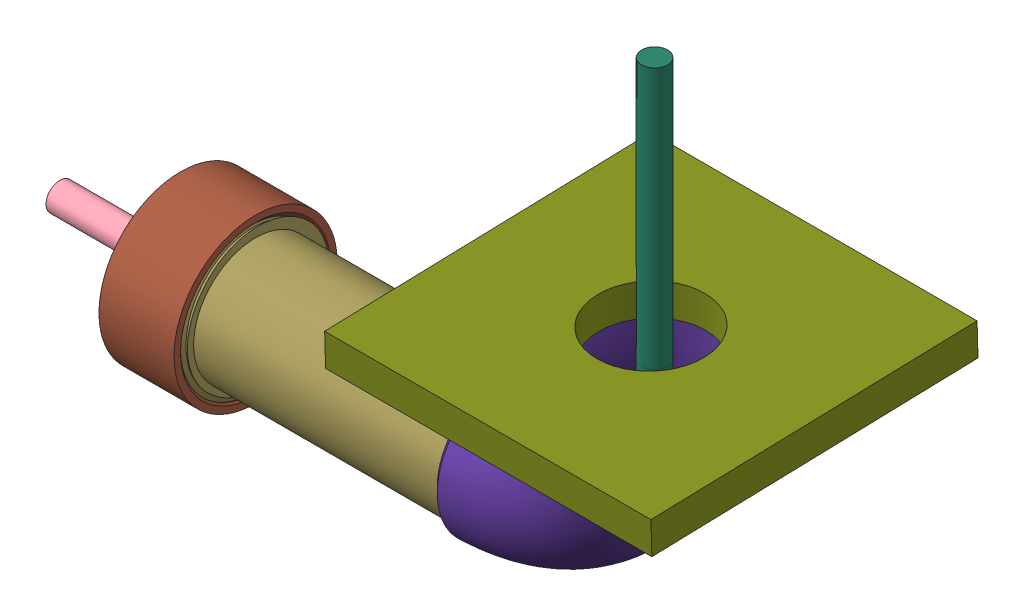
SolidWorks assembly new feedthrough 5, configuration Default. Lengths in mm.
Overall size (232.75 156.06 100.24).
30 component instances, 17 part files, 31 mates.
Components (placement in the parent):
- PCB-1: PCB [Default] at origin size (2 20 20)
- 1424177.stp-1: 1424177.stp [Default] at (6.35 0 0) x (0 -0.707107 0.707107) z (-1 0 0) size (27.6 26.9 24.95)
  - BS-BF-HW-BUCHSE-CAT6A_SW0001.stp-1: BS-BF-HW-BUCHSE-CAT6A_SW0001.stp [Default] at origin size (17.2 20.01 24.95)
  - 415371.stp-1: 415371.stp [Default] at (0 0 -8.45) x (-0.866025 -0.5 0) z (0 0 -1) size (20.9 19 2.8)
- cable assem-1: cable assem [Default] at (-53.2936 -50.2297 -9.5758) x (1 0 0) z (0 0.707107 0.707107) size (73.59 15.36 15.36)
  - cable-1: cable [Default] at (41.7936 28.7467 42.2889) x (0 0 1) z (-1 0 0) size (8.5 8.5 60.1)
  - 2 wires-1: 2 wires [Default] at (41.7936 28.7467 42.2889) x (0 1 0) z (1 0 0) size (5.09 5.18 13.49)
  - 2 wires-2: 2 wires [Default] at (41.7936 28.7467 42.2889) x (0 0 1) z (1 0 0) size (5.09 5.18 13.49)
  - 2 wires-3: 2 wires [Default] at (41.7936 28.7467 42.2889) x (0 -1 0) z (1 0 0) size (5.09 5.18 13.49)
  - 2 wires-4: 2 wires [Default] at (41.7936 28.7467 42.2889) x (0 0 -1) z (1 0 0) size (5.09 5.18 13.49)
- outer flange-2: outer flange [Default] at (-29 0 0) x (-1 0 0) z (0 0.99058 0.136937) size (28 41.9 41.9)
- end cap-1: end cap [Default] at (-17.5 0 0) x (1 0 0) z (0 0.006202 0.999981) size (4 12 12)
- end cap-2: end cap [Default] at (-43.5 0 0) x (-1 0 0) z (0 -0.926575 -0.37611) size (4 12 12)
- support plate-1: support plate [Default] at (11 0 0) x (0 0.797275 -0.603617) z (0 0.603617 0.797275) size (31 4 31)
- 92290A058_Super-Corrosion-Resistant 316 Stainless Steel Socket Head Screw-1: 92290A058_Super-Corrosion-Resistant 316 Stainless Steel Socket Head Screw [92290A058] at (3 10.3646 -7.847) x (0 0.578122 0.81595) z (-1 0 0) size (4.5 4.5 10.62)
- 93655A361_Male-Female Threaded Hex Standoff-1: 93655A361_Male-Female Threaded Hex Standoff [93655A361] at (-10.45 10.3646 -7.847) x (-1 0 0) z (0 0.711178 -0.703012) size (34.9 5.2 4.5)
- 92290A058_Super-Corrosion-Resistant 316 Stainless Steel Socket Head Screw-8: 92290A058_Super-Corrosion-Resistant 316 Stainless Steel Socket Head Screw [92290A058] at (3 7.847 10.3646) x (0 -0.81595 0.578122) z (-1 0 0) size (4.5 4.5 10.62)
- 92290A058_Super-Corrosion-Resistant 316 Stainless Steel Socket Head Screw-9: 92290A058_Super-Corrosion-Resistant 316 Stainless Steel Socket Head Screw [92290A058] at (3 -10.3646 7.847) x (0 -0.578122 -0.81595) z (-1 0 0) size (4.5 4.5 10.62)
- 92290A058_Super-Corrosion-Resistant 316 Stainless Steel Socket Head Screw-10: 92290A058_Super-Corrosion-Resistant 316 Stainless Steel Socket Head Screw [92290A058] at (3 -7.847 -10.3646) x (0 0.81595 -0.578122) z (-1 0 0) size (4.5 4.5 10.62)
- 93655A361_Male-Female Threaded Hex Standoff-8: 93655A361_Male-Female Threaded Hex Standoff [93655A361] at (-10.45 7.847 10.3646) x (-1 0 0) z (0 0.703012 0.711178) size (34.9 5.2 4.5)
- 93655A361_Male-Female Threaded Hex Standoff-9: 93655A361_Male-Female Threaded Hex Standoff [93655A361] at (-10.45 -10.3646 7.847) x (-1 0 0) z (0 -0.711178 0.703012) size (34.9 5.2 4.5)
- 93655A361_Male-Female Threaded Hex Standoff-10: 93655A361_Male-Female Threaded Hex Standoff [93655A361] at (-10.45 -7.847 -10.3646) x (-1 0 0) z (0 -0.703012 -0.711178) size (34.9 5.2 4.5)
- flange cover v3-1: flange cover v3 [Default] at (-34.5 0 0) x (0 0.999164 0.040884) z (0 0.040884 -0.999164) size (50 23.78 50)
- innder flange v2-1: innder flange v2 [Default] at (-26.5 0 0) x (0 0.988801 0.149242) z (0 0.149242 -0.988801) size (47.32 90.66 45)
- M12 cable-1: M12 cable [Default] at (12.9 0 0) x (-1 0 0) z (0 -0.986189 0.165625) size (101.9 33.14 134.89)
  - M12 cable a-1: M12 cable a [Default] at origin size (29.9 16 16)
  - M12 cable b-1: M12 cable b [Default] at (5 0 0) size (20 15 15)
  - 8mm cable v4-1: 8mm cable v4 [Default] at (-44.9 0 0) x (1 0 0) z (0 0.986189 -0.165625) size (57 132 8)
- plate-1: plate [Default] at (111.252 47.7334 1.3309) x (1 0 0) z (0 -0.027872 0.999612) size (100 10 100)
- 45555K514_Standard-Wall Butt-Weld Unthreaded Pipe Fitting-1: 45555K514_Standard-Wall Butt-Weld Unthreaded Pipe Fitting [45555K514] at (63.5 47.7334 1.3309) x (0 0.999612 0.027872) z (0 0.027872 -0.999612) size (69.01 69.01 42.36)
Mates (geometry in assembly coordinates):
- Concentric1: concentric aligned: cylinder of PCB-1 through (2 3.5355 3.5355) axis (-1 0 0) radius 0.5; cylinder of 1424177.stp-1/BS-BF-HW-BUCHSE-CAT6A_SW0001.stp-1 through (2 3.5355 3.5355) axis (-1 0 0) radius 0.5
- Concentric2: concentric aligned: cylinder of PCB-1 through (2 -3.5355 3.5355) axis (-1 0 0) radius 0.5; cylinder of 1424177.stp-1/BS-BF-HW-BUCHSE-CAT6A_SW0001.stp-1 through (2 -3.5355 3.5355) axis (-1 0 0) radius 0.5
- Coincident1: coincident anti-aligned: plane of 1424177.stp-1/BS-BF-HW-BUCHSE-CAT6A_SW0001.stp-1 through (2 0 0) normal (-1 0 0); plane of PCB-1 through (2 0 0) normal (1 0 0)
- Concentric3: concentric aligned: cylinder of cable assem-1/cable-1 through (-71.5 0 0) axis (1 0 0) radius 4.25; cylinder of outer flange-2 through (-29 0 0) axis (1 0 0) radius 4.25
- Distance1: distance = 5 mm aligned: plane of cable assem-1/cable-1 through (-11.5 0 0) normal (1 0 0); plane of outer flange-2 through (-16.5 0 0) normal (1 0 0)
- Concentric4: concentric anti-aligned: cylinder of outer flange-2 through (-29 0 0) axis (1 0 0) radius 6; cylinder of end cap-1 through (-15.5023 0 0) axis (-1 0 0) radius 5
- Coincident3: coincident aligned: plane of outer flange-2 through (-16.5 0 0) normal (1 0 0); plane of end cap-1 through (-16.5 0 0) normal (1 0 0)
- Concentric5: concentric aligned: cylinder of outer flange-2 through (-29 0 0) axis (1 0 0) radius 6; cylinder of end cap-2 through (-45.4977 0 0) axis (1 0 0) radius 5
- Coincident4: coincident aligned: plane of outer flange-2 through (-44.5 0 0) normal (-1 0 0); plane of end cap-2 through (-44.5 0 0) normal (-1 0 0)
- Concentric21: concentric anti-aligned: cylinder of PCB-1 through (2 0 0) axis (-1 0 0) radius 10; cylinder of support plate-1 through (7 0 0) axis (1 0 0) radius 7
- Coincident10: coincident anti-aligned: plane of 1424177.stp-1/BS-BF-HW-BUCHSE-CAT6A_SW0001.stp-1 through (7 0 0) normal (1 0 0); plane of support plate-1 through (7 0 0) normal (-1 0 0)
- Concentric22: concentric anti-aligned: cylinder of support plate-1 through (7 10.3646 -7.847) axis (1 0 0) radius 1.5; cylinder of 92290A058_Super-Corrosion-Resistant 316 Stainless Steel Socket Head Screw-1 through (11 10.3646 -7.847) axis (-1 0 0) radius 1.25
- Coincident11: coincident anti-aligned: plane of support plate-1 through (11 0 0) normal (1 0 0); circle of 92290A058_Super-Corrosion-Resistant 316 Stainless Steel Socket Head Screw-1
- Coincident18: coincident anti-aligned: plane of outer flange-2 through (-24 0 0) normal (1 0 0); plane of 93655A361_Male-Female Threaded Hex Standoff-1 through (-24 12.191 -5.9993) normal (-1 0 0)
- Concentric27: concentric aligned: cylinder of outer flange-2 through (-29 0 0) axis (1 0 0) radius 7; circle of flange cover-1
- Coincident20: coincident anti-aligned: plane of outer flange-2 through (-31.5 0 0) normal (-1 0 0); plane of flange cover-1 through (-31.5 0 0) normal (1 0 0)
- Concentric28: concentric aligned: cylinder of flange cover-1 through (-11.5 0 0) axis (-1 0 0) radius 25; cylinder of innder flange v2-1 through (15.5 0 0) axis (-1 0 0) radius 16.5
- Coincident22: coincident aligned: plane of flange cover-1 through (-11.5 0 0) normal (1 0 0); plane of innder flange v2-1 through (-11.5 0 0) normal (1 0 0)
- Concentric30: concentric anti-aligned: cylinder of outer flange-2 through (-29 -10.3646 7.847) axis (1 0 0) radius 1.25; cylinder of 93655A361_Male-Female Threaded Hex Standoff-9 through (-24 -10.3646 7.847) axis (-1 0 0) radius 1.25
- Concentric31: concentric anti-aligned: cylinder of outer flange-2 through (-29 -7.847 -10.3646) axis (1 0 0) radius 1.25; cylinder of 93655A361_Male-Female Threaded Hex Standoff-10 through (-24 -7.847 -10.3646) axis (-1 0 0) radius 1.25
- Concentric32: concentric aligned: circle of 1424177.stp-1/BS-BF-HW-BUCHSE-CAT6A_SW0001.stp-1; circle of M12 cable-1/M12 cable a-1
- Coincident24: coincident anti-aligned: plane of 1424177.stp-1/BS-BF-HW-BUCHSE-CAT6A_SW0001.stp-1 through (23 0 0) normal (1 0 0); plane of M12 cable-1/M12 cable a-1 through (23 -1.0434 -6.213) normal (-1 0 0)
- Coincident25: coincident: line of M12 cable-1/8mm cable-1 through (110.8 48 0) axis (0 1 0)
- Parallel1: parallel anti-aligned: plane of plate-1 through (61.252 57.7296 1.6096) normal (-1 0 0)
- Concentric34: concentric anti-aligned: cylinder of 92290A058_Super-Corrosion-Resistant 316 Stainless Steel Socket Head Screw-8 through (11 7.847 10.3646) axis (-1 0 0) radius 1.25; cylinder of 93655A361_Male-Female Threaded Hex Standoff-8 through (2.2 7.847 10.3646) axis (1 0 0) radius 1.25
- Concentric35: concentric anti-aligned: cylinder of 92290A058_Super-Corrosion-Resistant 316 Stainless Steel Socket Head Screw-1 through (11 10.3646 -7.847) axis (-1 0 0) radius 1.25; cylinder of 93655A361_Male-Female Threaded Hex Standoff-1 through (2.2 10.3646 -7.847) axis (1 0 0) radius 1.25
- Coincident31: coincident anti-aligned: plane of support plate-1 through (7 0 0) normal (-1 0 0); plane of 93655A361_Male-Female Threaded Hex Standoff-1 through (7 12.191 -5.9993) normal (1 0 0)
- Concentric36: concentric aligned: circle of plate-1; circle of 45555K514_Standard-Wall Butt-Weld Unthreaded Pipe Fitting-1
- Coincident32: coincident anti-aligned: plane of plate-1 through (111.252 47.7334 1.3309) normal (0 -0.999612 -0.027872); plane of 45555K514_Standard-Wall Butt-Weld Unthreaded Pipe Fitting-1 through (111.252 47.7334 1.3309) normal (0 0.999612 0.027872)
- Concentric39: concentric aligned: cylinder of support plate-1 through (7 0 0) axis (1 0 0) radius 15.5; circle of 45555K514_Standard-Wall Butt-Weld Unthreaded Pipe Fitting-1
- Coincident34: coincident anti-aligned: plane of innder flange v2-1 through (63.5 0 0) normal (1 0 0); plane of 45555K514_Standard-Wall Butt-Weld Unthreaded Pipe Fitting-1 through (63.5 0 0) normal (-1 0 0)
